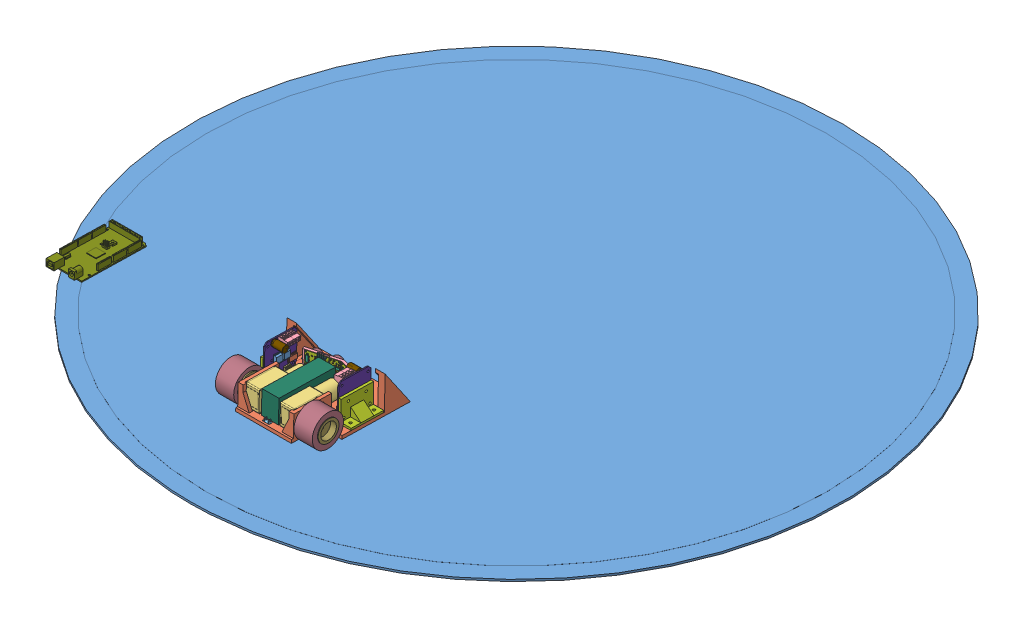
SolidWorks assembly Assem1, configuration Default. Lengths in mm.
Overall size (1000 206.44 1000).
164 component instances, 79 part files, 2 mates.
Components (placement in the parent):
- 0.Sân-1: 0.Sân [Default] at (-54.2257 -2.4148 29.2017) size (1000 3.1 1000)
- 00.ver1-1: 00.ver1 [Default] at (-231.8251 -97.2904 292.0916) x (-0.002357 -0.023857 -0.999713) z (0.999997 0 -0.002358) size (730.91 273.09 435.6)
  - 1.De-1: 1.De [Default] at (-19.2301 99.4537 139.4255) size (150 55.06 150)
  - 4.JGY370_Reduction DC Motor-6mm-1: 4.JGY370_Reduction DC Motor-6mm [Default] at (-65.2301 120.4537 174.9255) x (1 0 0) z (0 -1 0) size (80.2 40.2 32)
  - 4.JGY370_Reduction DC Motor-6mm-2: 4.JGY370_Reduction DC Motor-6mm [Default] at (-65.2301 120.4537 103.9255) x (1 0 0) z (0 1 0) size (80.2 40.2 32)
  - Assem5-1: Assem5 [Default] at (96.0425 162.0175 178.5362) x (0 0 -1) z (-1 0 0) size (428.08 57.86 515.26)
    - 11.Ga_sieu_am-1: 11.Ga_sieu_am [Default] at (39.1106 32.5638 61.7658) size (96.59 25 29.76)
    - 6. HC-04HC-04.stp-1: 6. HC-04HC-04.stp [Default] at (61.5511 42.5638 72.9551) x (-0.965926 0 -0.258819) z (0.258819 0 -0.965926) size (45 25.57 17.46)
      - HC-04Array.stp-1: HC-04Array.stp [Default] at origin size (10.16 2.54 2.54)
      - HC-04Array001.stp-1: HC-04Array001.stp [Default] at (0 0 1) size (8.32 7.52 6.46)
      - HC-04Placa.stp-1: HC-04Placa.stp [Default] at origin size (45 20 1)
      - HC-04Pad003.stp-1: HC-04Pad003.stp [Default] at (0 0 1) size (10.52 3.38 0.2)
      - HC-04Fillet.stp-1: HC-04Fillet.stp [Default] at (0 0 1) size (10.1 2.84 3)
      - HC-04Array002.stp-1: HC-04Array002.stp [Default] at origin size (9.62 2 1)
      - HC-04Array003.stp-1: HC-04Array003.stp [Default] at (0 0 1) size (28 12 0.8)
      - HC-04Fusion.stp-1: HC-04Fusion.stp [Default] at origin size (6 2 1)
      - HC-04Fillet001.stp-1: HC-04Fillet001.stp [Default] at (0 0 1) size (42 16 12)
      - HC-04Pad005.stp-1: HC-04Pad005.stp [Default] at (0 0 1) size (39.16 13 0.2)
      - HC-04Pad006.stp-1: HC-04Pad006.stp [Default] at (0 0 1) size (35.01 9.04 7)
      - HC-04Fusion001.stp-1: HC-04Fusion001.stp [Default] at (0 0 8) size (31 5 1.5)
      - HC-04Clone_of_Fusion002.stp-1: HC-04Clone_of_Fusion002.stp [Default] at (47.2 -5.5 12.6) size (13 13 0.15)
      - HC-04Clone_of_Fusion003.stp-1: HC-04Clone_of_Fusion003.stp [Default] at (21.2 -5.5 12.6) size (13 13 0.15)
      - HC-04Array005.stp-1: HC-04Array005.stp [Default] at origin size (9.62 2 1)
      - HC-04Array002002.stp-1: HC-04Array002002.stp [Default] at (-5.9 0.1 0.15) size (6.57 1.4 0.56)
      - HC-04Clone_of_Array002002.stp-1: HC-04Clone_of_Array002002.stp [Default] at (-23.9 0.1 0.15) size (6.57 1.4 0.56)
      - HC-04Array002003.stp-1: HC-04Array002003.stp [Default] at (-6.05 0 0.15) size (6.57 1.4 0.56)
      - HC-04Clone_of_Array002003.stp-1: HC-04Clone_of_Array002003.stp [Default] at (-24.05 0 0.15) size (6.57 1.4 0.56)
      - HC-04Integrados.stp-1: HC-04Integrados.stp [Default] at origin size (42.14 9 1)
      - HC-04ShapeString.stp-1: HC-04ShapeString.stp [Default] at (-3.2 -7 1.01) x (0 1 0) z (0 0 1) size (2.53 1.13 0.01)
      - HC-04ShapeString001.stp-1: HC-04ShapeString001.stp [Default] at (-0.6 -7 1.01) x (0 1 0) z (0 0 1) size (2.66 1.45 0.01)
      - HC-04ShapeString002.stp-1: HC-04ShapeString002.stp [Default] at (1.9 -7 1.01) x (0 1 0) z (0 0 1) size (3.21 1.16 0.01)
      - HC-04ShapeString003.stp-1: HC-04ShapeString003.stp [Default] at (4.5 -7 1.01) x (0 1 0) z (0 0 1) size (2.71 1.16 0.01)
      - HC-04ShapeString004.stp-1: HC-04ShapeString004.stp [Default] at (-19.5 -9.3 1.01) size (1.84 2.34 0.01)
      - HC-04ShapeString005.stp-1: HC-04ShapeString005.stp [Default] at (17.5 -9.3 1.01) size (1.82 2.34 0.01)
      - HC-04ShapeString006.stp-1: HC-04ShapeString006.stp [Default] at (-3 3.7 1.01) size (5.52 1.41 0.01)
      - HC-04Pad008.stp-1: HC-04Pad008.stp [Default] at (0 0 -0.01) size (44.56 19.6 1.02)
      - HC-04Scale004.stp-1: HC-04Scale004.stp [Default] at (-1.9 -21.5 -1.5) x (0 1 0) z (0 0 1) size (0.8 1.77 0.5)
      - HC-04Scale027.stp-1: HC-04Scale027.stp [Default] at (-1.9 -10.2323 -1.5) x (0 1 0) z (0 0 1) size (0.8 1.77 0.5)
      - HC-04Scale028.stp-1: HC-04Scale028.stp [Default] at (8.5984 -21.5 -1.5) x (0 1 0) z (0 0 1) size (0.8 1.77 0.5)
      - HC-04Scale029.stp-1: HC-04Scale029.stp [Default] at (8.5984 -19.5867 -1.5) x (0 1 0) z (0 0 1) size (0.8 1.77 0.5)
      - HC-04Scale030.stp-1: HC-04Scale030.stp [Default] at (8.5984 -17.5982 -1.5) x (0 1 0) z (0 0 1) size (0.8 1.77 0.5)
      - HC-04Scale031.stp-1: HC-04Scale031.stp [Default] at (8.5984 -15.6427 -1.5) x (0 1 0) z (0 0 1) size (0.8 1.77 0.5)
      - HC-04Scale032.stp-1: HC-04Scale032.stp [Default] at (8.5984 -11.6848 -1.5) x (0 1 0) z (0 0 1) size (0.8 1.77 0.5)
      - HC-04Scale033.stp-1: HC-04Scale033.stp [Default] at (-26.74 -2 -1.5) x (0 1 0) z (0 0 1) size (0.8 1.85 0.5)
      - HC-04Scale034.stp-1: HC-04Scale034.stp [Default] at (24.9371 -21.5 -1.5) x (0 1 0) z (0 0 1) size (0.8 1.77 0.5)
      - HC-04Scale035.stp-1: HC-04Scale035.stp [Default] at (24.9691 -19.5867 -1.5) x (0 1 0) z (0 0 1) size (0.8 1.77 0.5)
      - HC-04Scale036.stp-1: HC-04Scale036.stp [Default] at (24.9742 -17.5982 -1.5) x (0 1 0) z (0 0 1) size (0.8 1.77 0.5)
      - HC-04Scale037.stp-1: HC-04Scale037.stp [Default] at (-10.4013 -2 -1.5) x (0 1 0) z (0 0 1) size (0.8 1.85 0.5)
      - HC-04Scale038.stp-1: HC-04Scale038.stp [Default] at (-10.4013 -3.9266 -1.5) x (0 1 0) z (0 0 1) size (0.8 1.85 0.5)
      - HC-04Scale039.stp-1: HC-04Scale039.stp [Default] at (-10.4013 -0.0734 -1.5) x (0 1 0) z (0 0 1) size (0.8 1.85 0.5)
      - HC-04Scale040.stp-1: HC-04Scale040.stp [Default] at (24.9742 -9.855 -1.5) x (0 1 0) z (0 0 1) size (0.8 1.77 0.5)
      - HC-04Scale041.stp-1: HC-04Scale041.stp [Default] at (26.5673 -24.0564 -1.5) x (0 1 0) z (0 0 1) size (0.8 1.77 0.5)
      - HC-04Scale042.stp-1: HC-04Scale042.stp [Default] at (26.5673 -7.3333 -1.5) x (0 1 0) z (0 0 1) size (0.8 1.77 0.5)
      - HC-04Scale043.stp-1: HC-04Scale043.stp [Default] at (30.1435 -7.3333 -1.5) x (0 1 0) z (0 0 1) size (0.8 1.77 0.5)
      - HC-04Scale044.stp-1: HC-04Scale044.stp [Default] at (33.5459 -7.3333 -1.5) x (0 1 0) z (0 0 1) size (0.8 1.77 0.5)
      - HC-04Scale045.stp-1: HC-04Scale045.stp [Default] at (37.7181 -11.1827 -1.5) x (0 1 0) z (0 0 1) size (0.8 1.77 0.5)
      - HC-04Scale046.stp-1: HC-04Scale046.stp [Default] at (37.7181 -20.5932 -1.5) x (0 1 0) z (0 0 1) size (0.8 1.77 0.5)
      - HC-04Scale047.stp-1: HC-04Scale047.stp [Default] at (-3.9042 -12.3288 -1.5) x (0 1 0) z (0 0 1) size (0.8 1.85 0.5)
      - HC-04Scale048.stp-1: HC-04Scale048.stp [Default] at (13.5402 13.2894 -1.5) size (0.8 1.85 0.5)
      - HC-04Scale049.stp-1: HC-04Scale049.stp [Default] at (13.5402 23.7909 -1.5) size (0.8 1.85 0.5)
      - HC-04Pad009.stp-1: HC-04Pad009.stp [Default] x (1 0 0) z (0 0 -1) size (42.21 18.43 0.01)
      - HC-04ShapeString007.stp-1: HC-04ShapeString007.stp [Default] at (-3.2 -7 -0.1) x (0 1 0) z (0 0 1) size (2.53 1.13 0.01)
      - HC-04ShapeString008.stp-1: HC-04ShapeString008.stp [Default] at (-0.6 -7 -0.1) x (0 1 0) z (0 0 1) size (2.66 1.45 0.01)
      - HC-04ShapeString009.stp-1: HC-04ShapeString009.stp [Default] at (1.9 -7 -0.1) x (0 1 0) z (0 0 1) size (3.21 1.16 0.01)
      - HC-04ShapeString010.stp-1: HC-04ShapeString010.stp [Default] at (4.5 -7 -0.1) x (0 1 0) z (0 0 1) size (2.71 1.16 0.01)
      - HC-04Fusion002.stp-1: HC-04Fusion002.stp [Default] at origin size (5.7 7.57 0.56)
      - HC-04ShapeString011.stp-1: HC-04ShapeString011.stp [Default] at (-17.5 8.4 1.1) size (7.91 1.16 0.01)
      - HC-04ShapeString012.stp-1: HC-04ShapeString012.stp [Default] at (-7.5 8 -0.1) x (-1 0 0) z (0 0 -1) size (7.91 1.16 0.01)
    - 6. HC-04HC-04.stp-2: 6. HC-04HC-04.stp [Default] at (16.6702 42.5638 72.9551) x (-0.965926 0 0.258819) z (-0.258819 0 -0.965926) size (45 25.57 17.46)
      - HC-04Array.stp-1: HC-04Array.stp [Default] at origin size (10.16 2.54 2.54)
      - HC-04Array001.stp-1: HC-04Array001.stp [Default] at (0 0 1) size (8.32 7.52 6.46)
      - HC-04Placa.stp-1: HC-04Placa.stp [Default] at origin size (45 20 1)
      - HC-04Pad003.stp-1: HC-04Pad003.stp [Default] at (0 0 1) size (10.52 3.38 0.2)
      - HC-04Fillet.stp-1: HC-04Fillet.stp [Default] at (0 0 1) size (10.1 2.84 3)
      - HC-04Array002.stp-1: HC-04Array002.stp [Default] at origin size (9.62 2 1)
      - HC-04Array003.stp-1: HC-04Array003.stp [Default] at (0 0 1) size (28 12 0.8)
      - HC-04Fusion.stp-1: HC-04Fusion.stp [Default] at origin size (6 2 1)
      - HC-04Fillet001.stp-1: HC-04Fillet001.stp [Default] at (0 0 1) size (42 16 12)
      - HC-04Pad005.stp-1: HC-04Pad005.stp [Default] at (0 0 1) size (39.16 13 0.2)
      - HC-04Pad006.stp-1: HC-04Pad006.stp [Default] at (0 0 1) size (35.01 9.04 7)
      - HC-04Fusion001.stp-1: HC-04Fusion001.stp [Default] at (0 0 8) size (31 5 1.5)
      - HC-04Clone_of_Fusion002.stp-1: HC-04Clone_of_Fusion002.stp [Default] at (47.2 -5.5 12.6) size (13 13 0.15)
      - HC-04Clone_of_Fusion003.stp-1: HC-04Clone_of_Fusion003.stp [Default] at (21.2 -5.5 12.6) size (13 13 0.15)
      - HC-04Array005.stp-1: HC-04Array005.stp [Default] at origin size (9.62 2 1)
      - HC-04Array002002.stp-1: HC-04Array002002.stp [Default] at (-5.9 0.1 0.15) size (6.57 1.4 0.56)
      - HC-04Clone_of_Array002002.stp-1: HC-04Clone_of_Array002002.stp [Default] at (-23.9 0.1 0.15) size (6.57 1.4 0.56)
      - HC-04Array002003.stp-1: HC-04Array002003.stp [Default] at (-6.05 0 0.15) size (6.57 1.4 0.56)
      - HC-04Clone_of_Array002003.stp-1: HC-04Clone_of_Array002003.stp [Default] at (-24.05 0 0.15) size (6.57 1.4 0.56)
      - HC-04Integrados.stp-1: HC-04Integrados.stp [Default] at origin size (42.14 9 1)
      - HC-04ShapeString.stp-1: HC-04ShapeString.stp [Default] at (-3.2 -7 1.01) x (0 1 0) z (0 0 1) size (2.53 1.13 0.01)
      - HC-04ShapeString001.stp-1: HC-04ShapeString001.stp [Default] at (-0.6 -7 1.01) x (0 1 0) z (0 0 1) size (2.66 1.45 0.01)
      - HC-04ShapeString002.stp-1: HC-04ShapeString002.stp [Default] at (1.9 -7 1.01) x (0 1 0) z (0 0 1) size (3.21 1.16 0.01)
      - HC-04ShapeString003.stp-1: HC-04ShapeString003.stp [Default] at (4.5 -7 1.01) x (0 1 0) z (0 0 1) size (2.71 1.16 0.01)
      - HC-04ShapeString004.stp-1: HC-04ShapeString004.stp [Default] at (-19.5 -9.3 1.01) size (1.84 2.34 0.01)
      - HC-04ShapeString005.stp-1: HC-04ShapeString005.stp [Default] at (17.5 -9.3 1.01) size (1.82 2.34 0.01)
      - HC-04ShapeString006.stp-1: HC-04ShapeString006.stp [Default] at (-3 3.7 1.01) size (5.52 1.41 0.01)
      - HC-04Pad008.stp-1: HC-04Pad008.stp [Default] at (0 0 -0.01) size (44.56 19.6 1.02)
      - HC-04Scale004.stp-1: HC-04Scale004.stp [Default] at (-1.9 -21.5 -1.5) x (0 1 0) z (0 0 1) size (0.8 1.77 0.5)
      - HC-04Scale027.stp-1: HC-04Scale027.stp [Default] at (-1.9 -10.2323 -1.5) x (0 1 0) z (0 0 1) size (0.8 1.77 0.5)
      - HC-04Scale028.stp-1: HC-04Scale028.stp [Default] at (8.5984 -21.5 -1.5) x (0 1 0) z (0 0 1) size (0.8 1.77 0.5)
      - HC-04Scale029.stp-1: HC-04Scale029.stp [Default] at (8.5984 -19.5867 -1.5) x (0 1 0) z (0 0 1) size (0.8 1.77 0.5)
      - HC-04Scale030.stp-1: HC-04Scale030.stp [Default] at (8.5984 -17.5982 -1.5) x (0 1 0) z (0 0 1) size (0.8 1.77 0.5)
      - HC-04Scale031.stp-1: HC-04Scale031.stp [Default] at (8.5984 -15.6427 -1.5) x (0 1 0) z (0 0 1) size (0.8 1.77 0.5)
      - HC-04Scale032.stp-1: HC-04Scale032.stp [Default] at (8.5984 -11.6848 -1.5) x (0 1 0) z (0 0 1) size (0.8 1.77 0.5)
      - HC-04Scale033.stp-1: HC-04Scale033.stp [Default] at (-26.74 -2 -1.5) x (0 1 0) z (0 0 1) size (0.8 1.85 0.5)
      - HC-04Scale034.stp-1: HC-04Scale034.stp [Default] at (24.9371 -21.5 -1.5) x (0 1 0) z (0 0 1) size (0.8 1.77 0.5)
      - HC-04Scale035.stp-1: HC-04Scale035.stp [Default] at (24.9691 -19.5867 -1.5) x (0 1 0) z (0 0 1) size (0.8 1.77 0.5)
      - HC-04Scale036.stp-1: HC-04Scale036.stp [Default] at (24.9742 -17.5982 -1.5) x (0 1 0) z (0 0 1) size (0.8 1.77 0.5)
      - HC-04Scale037.stp-1: HC-04Scale037.stp [Default] at (-10.4013 -2 -1.5) x (0 1 0) z (0 0 1) size (0.8 1.85 0.5)
      - HC-04Scale038.stp-1: HC-04Scale038.stp [Default] at (-10.4013 -3.9266 -1.5) x (0 1 0) z (0 0 1) size (0.8 1.85 0.5)
      - HC-04Scale039.stp-1: HC-04Scale039.stp [Default] at (-10.4013 -0.0734 -1.5) x (0 1 0) z (0 0 1) size (0.8 1.85 0.5)
      - HC-04Scale040.stp-1: HC-04Scale040.stp [Default] at (24.9742 -9.855 -1.5) x (0 1 0) z (0 0 1) size (0.8 1.77 0.5)
      - HC-04Scale041.stp-1: HC-04Scale041.stp [Default] at (26.5673 -24.0564 -1.5) x (0 1 0) z (0 0 1) size (0.8 1.77 0.5)
      - HC-04Scale042.stp-1: HC-04Scale042.stp [Default] at (26.5673 -7.3333 -1.5) x (0 1 0) z (0 0 1) size (0.8 1.77 0.5)
      - HC-04Scale043.stp-1: HC-04Scale043.stp [Default] at (30.1435 -7.3333 -1.5) x (0 1 0) z (0 0 1) size (0.8 1.77 0.5)
      - HC-04Scale044.stp-1: HC-04Scale044.stp [Default] at (33.5459 -7.3333 -1.5) x (0 1 0) z (0 0 1) size (0.8 1.77 0.5)
      - HC-04Scale045.stp-1: HC-04Scale045.stp [Default] at (37.7181 -11.1827 -1.5) x (0 1 0) z (0 0 1) size (0.8 1.77 0.5)
      - HC-04Scale046.stp-1: HC-04Scale046.stp [Default] at (37.7181 -20.5932 -1.5) x (0 1 0) z (0 0 1) size (0.8 1.77 0.5)
      - HC-04Scale047.stp-1: HC-04Scale047.stp [Default] at (-3.9042 -12.3288 -1.5) x (0 1 0) z (0 0 1) size (0.8 1.85 0.5)
      - HC-04Scale048.stp-1: HC-04Scale048.stp [Default] at (13.5402 13.2894 -1.5) size (0.8 1.85 0.5)
      - HC-04Scale049.stp-1: HC-04Scale049.stp [Default] at (13.5402 23.7909 -1.5) size (0.8 1.85 0.5)
      - HC-04Pad009.stp-1: HC-04Pad009.stp [Default] x (1 0 0) z (0 0 -1) size (42.21 18.43 0.01)
      - HC-04ShapeString007.stp-1: HC-04ShapeString007.stp [Default] at (-3.2 -7 -0.1) x (0 1 0) z (0 0 1) size (2.53 1.13 0.01)
      - HC-04ShapeString008.stp-1: HC-04ShapeString008.stp [Default] at (-0.6 -7 -0.1) x (0 1 0) z (0 0 1) size (2.66 1.45 0.01)
      - HC-04ShapeString009.stp-1: HC-04ShapeString009.stp [Default] at (1.9 -7 -0.1) x (0 1 0) z (0 0 1) size (3.21 1.16 0.01)
      - HC-04ShapeString010.stp-1: HC-04ShapeString010.stp [Default] at (4.5 -7 -0.1) x (0 1 0) z (0 0 1) size (2.71 1.16 0.01)
      - HC-04Fusion002.stp-1: HC-04Fusion002.stp [Default] at origin size (5.7 7.57 0.56)
      - HC-04ShapeString011.stp-1: HC-04ShapeString011.stp [Default] at (-17.5 8.4 1.1) size (7.91 1.16 0.01)
      - HC-04ShapeString012.stp-1: HC-04ShapeString012.stp [Default] at (-7.5 8 -0.1) x (-1 0 0) z (0 0 -1) size (7.91 1.16 0.01)
    - 12.ganh-1: 12.ganh [Default] at (59.9982 46.6638 78.7506) x (0.965926 0 0.258819) z (0 1 0) size (10 5 19)
    - 12.ganh-2: 12.ganh [Default] at (18.2231 46.6638 78.7506) x (0.965926 0 -0.258819) z (0 1 0) size (10 5 19)
  - 14.banhxe-2: 14.banhxe [Default] at (-87.2567 105.5442 114.1562) x (0 0 -1) z (0.914362 -0.404898 0) size (34 67.44 67.44)
    - 13.LoiBanhVer2-1: 13.LoiBanhVer2 [Default] at (34.7306 22.5513 14.1035) size (31 36 36)
    - 2.lop_banh_xe-1: 2.lop_banh_xe [Default] at (20.7306 22.5513 14.1035) x (0 -0.621853 -0.783134) z (1 0 0) size (48 48 28)
    - 3.Noi_truc-phi5-1: 3.Noi_truc-phi5 [Default] at (33.7306 22.5513 14.1035) x (0 0 1) z (0 -1 0) size (13.86 18 12)
  - 14.banhxe-3: 14.banhxe [Default] at (-86.3615 104.3004 164.6949) x (0 0 1) z (-0.093648 0.995605 0) size (34 67.44 67.44)
    - 13.LoiBanhVer2-1: 13.LoiBanhVer2 [Default] at (34.7306 22.5513 14.1035) size (31 36 36)
    - 2.lop_banh_xe-1: 2.lop_banh_xe [Default] at (20.7306 22.5513 14.1035) x (0 -0.621853 -0.783134) z (1 0 0) size (48 48 28)
    - 3.Noi_truc-phi5-1: 3.Noi_truc-phi5 [Default] at (33.7306 22.5513 14.1035) x (0 0 1) z (0 -1 0) size (13.86 18 12)
  - 9.pin-1: 9.pin [Default] at (-79.5165 121.9537 139.4255) x (0 1 0) z (1 0 0) size (35 26 87)
  - 7.Mega.step-1: 7.Mega.step [Default] at (-152.3386 260.2948 -55.459) size (109.6 12.5 53.34)
  - 8.BTS7960 43A HIGH POWER H BRIDGE MODULE-1: 8.BTS7960 43A HIGH POWER H BRIDGE MODULE [Default] at (-5.3451 132.3537 194.4255) x (-1 0 0) z (0 -1 0) size (49.5 20.8 49.96)
    - PCB, BTS7960 43A HIGH POWER H BRIDGE MODULE-1: PCB, BTS7960 43A HIGH POWER H BRIDGE MODULE [Default] at origin size (49.5 1.7 49.8)
    - ALUMINUM ELECTROLYTIC CAPACITOR, 330 uF, BTS7960 43A HIGH POWER H BRIDGE MODULE-1: ALUMINUM ELECTROLYTIC CAPACITOR, 330 uF, BTS7960 43A HIGH POWER H BRIDGE MODULE [Default] at (-10.75 1.8 -19.85) x (0.999469 0 -0.032584) z (0.032584 0 0.999469) size (10.1 18.7 10.1)
    - BTN7960 IC, BTS7960 43A HIGH POWER H BRIDGE MODULE-1: BTN7960 IC, BTS7960 43A HIGH POWER H BRIDGE MODULE [Default] at (5.95 1.7 1.8) x (-1 0 0) z (0 0 -1) size (9.6 4.6 14.9)
    - BTN7960 IC, BTS7960 43A HIGH POWER H BRIDGE MODULE-2: BTN7960 IC, BTS7960 43A HIGH POWER H BRIDGE MODULE [Default] at (-5.95 1.7 1.8) x (-1 0 0) z (0 0 -1) size (9.6 4.6 14.9)
    - NXP 74HC244D, BUFFER AND LINE DRIVER, BTS7960 43A HIGH POWER H BRIDGE MODULE-1: NXP 74HC244D, BUFFER AND LINE DRIVER, BTS7960 43A HIGH POWER H BRIDGE MODULE [Default] at (17.35 3 12.1) size (13 2.6 10.4)
    - y 8 PIN HEADER, IC, BTS7960 43A HIGH POWER H BRIDGE MODULE-1: y 8 PIN HEADER, IC, BTS7960 43A HIGH POWER H BRIDGE MODULE [Default] at (-34.78 4.2 20.29) x (0 0 -1) z (-1 0 0) size (5.08 11.6 10.16)
    - EUROSTYLE TERMINAL BLOCK 2 POS 5.0 MM RA PLUG, BTS7960 43A HIGH POWER H BRIDGE MODULE-1: EUROSTYLE TERMINAL BLOCK 2 POS 5.0 MM RA PLUG, BTS7960 43A HIGH POWER H BRIDGE MODULE [Default] at (0.75 4.2 -6.5) size (10 14.5 10.5)
    - EUROSTYLE TERMINAL BLOCK 2 POS 5.0 MM RA PLUG, BTS7960 43A HIGH POWER H BRIDGE MODULE-2: EUROSTYLE TERMINAL BLOCK 2 POS 5.0 MM RA PLUG, BTS7960 43A HIGH POWER H BRIDGE MODULE [Default] at (10.75 4.2 -6.5) size (10 14.5 10.5)
  - 8.BTS7960 43A HIGH POWER H BRIDGE MODULE-2: 8.BTS7960 43A HIGH POWER H BRIDGE MODULE [Default] at (-10.1468 132.3537 84.4255) x (1 0 0) z (0 -1 0) size (49.5 20.8 49.96)
    - PCB, BTS7960 43A HIGH POWER H BRIDGE MODULE-1: PCB, BTS7960 43A HIGH POWER H BRIDGE MODULE [Default] at origin size (49.5 1.7 49.8)
    - ALUMINUM ELECTROLYTIC CAPACITOR, 330 uF, BTS7960 43A HIGH POWER H BRIDGE MODULE-1: ALUMINUM ELECTROLYTIC CAPACITOR, 330 uF, BTS7960 43A HIGH POWER H BRIDGE MODULE [Default] at (-10.75 1.8 -19.85) x (0.999469 0 -0.032584) z (0.032584 0 0.999469) size (10.1 18.7 10.1)
    - BTN7960 IC, BTS7960 43A HIGH POWER H BRIDGE MODULE-1: BTN7960 IC, BTS7960 43A HIGH POWER H BRIDGE MODULE [Default] at (5.95 1.7 1.8) x (-1 0 0) z (0 0 -1) size (9.6 4.6 14.9)
    - BTN7960 IC, BTS7960 43A HIGH POWER H BRIDGE MODULE-2: BTN7960 IC, BTS7960 43A HIGH POWER H BRIDGE MODULE [Default] at (-5.95 1.7 1.8) x (-1 0 0) z (0 0 -1) size (9.6 4.6 14.9)
    - NXP 74HC244D, BUFFER AND LINE DRIVER, BTS7960 43A HIGH POWER H BRIDGE MODULE-1: NXP 74HC244D, BUFFER AND LINE DRIVER, BTS7960 43A HIGH POWER H BRIDGE MODULE [Default] at (17.35 3 12.1) size (13 2.6 10.4)
    - y 8 PIN HEADER, IC, BTS7960 43A HIGH POWER H BRIDGE MODULE-1: y 8 PIN HEADER, IC, BTS7960 43A HIGH POWER H BRIDGE MODULE [Default] at (-34.78 4.2 20.29) x (0 0 -1) z (-1 0 0) size (5.08 11.6 10.16)
    - EUROSTYLE TERMINAL BLOCK 2 POS 5.0 MM RA PLUG, BTS7960 43A HIGH POWER H BRIDGE MODULE-1: EUROSTYLE TERMINAL BLOCK 2 POS 5.0 MM RA PLUG, BTS7960 43A HIGH POWER H BRIDGE MODULE [Default] at (0.75 4.2 -6.5) size (10 14.5 10.5)
    - EUROSTYLE TERMINAL BLOCK 2 POS 5.0 MM RA PLUG, BTS7960 43A HIGH POWER H BRIDGE MODULE-2: EUROSTYLE TERMINAL BLOCK 2 POS 5.0 MM RA PLUG, BTS7960 43A HIGH POWER H BRIDGE MODULE [Default] at (10.75 4.2 -6.5) size (10 14.5 10.5)
  - 10.1.TCRT5000mod-1: 10.1.TCRT5000mod [Default] at (-60.9052 110.0625 132.4255) x (0.526489 -0.850182 0) z (0 0 1) size (10.63 8.2 10)
  - 10.1.TCRT5000mod-2: 10.1.TCRT5000mod [Default] at (70.0948 112.0625 132.4255) x (0.526489 -0.850182 0) z (0 0 1) size (10.63 8.2 10)
  - 10.2.TCRT5000mod-1: 10.2.TCRT5000mod [Default] at (24.6562 106.0625 96.6621) x (-0.261635 -0.850182 -0.456879) z (0.867784 0 -0.496942) size (17.6 34.23 14)
  - 14.Ga_BTS-3: 14.Ga_BTS [Default] at (19.7549 104.4537 194.4255) x (0 0 1) z (-1 0 0) size (20 33 50)
  - 14.Ga_BTS-4: 14.Ga_BTS [Default] at (-35.2468 104.4537 84.4255) x (0 0 -1) z (1 0 0) size (20 33 50)
Mates (geometry in assembly coordinates):
- Tangent1: tangent anti-aligned: plane of 0.Sân-1 through (-54.2257 0.6852 29.2017) normal (0 1 0); cylinder of 00.ver1-1/14.banhxe-3/2.lop_banh_xe-1 through (-18.2531 24.6852 353.926) axis (-0.999997 0 0.002358) radius 24
- Coincident1: coincident: plane of 0.Sân-1 through (-54.2257 0.6852 29.2017) normal (0 1 0); line of 00.ver1-1/1.De-1 through (-17.549 0.6852 228.4608) axis (-0.999997 0 0.002358)
